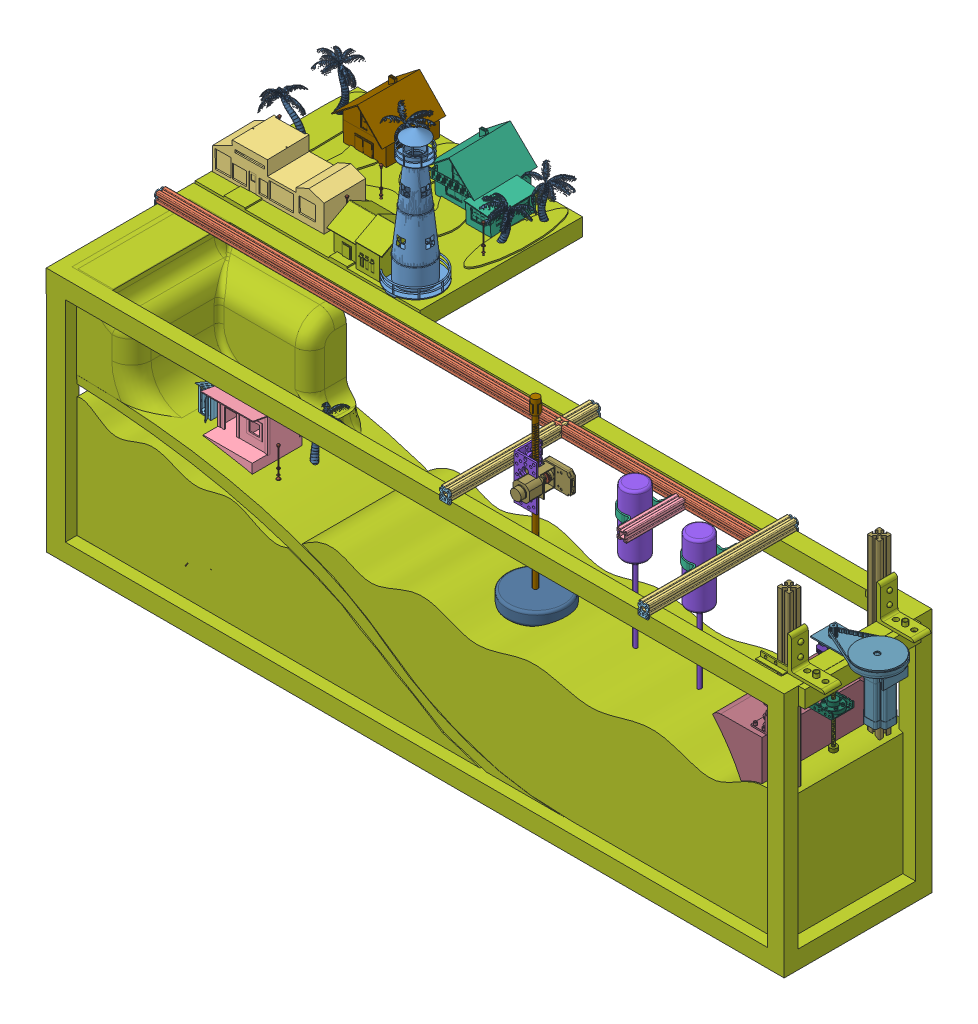
SolidWorks assembly Final SIWEED Town, configuration Default. Lengths in mm.
Overall size (1624.1 772.82 662.75).
56 component instances, 30 part files, 0 mates.
Components (placement in the parent):
- light house-1: light house [Valor predeterminado] at (-330.237 25.4911 -51.0609) size (102.96 270.27 102.96)
- tubular-seaweed-kcasal-2: tubular-seaweed-kcasal [Default] at (-568.4367 -469.1582 111.9112) size (107.7 163.84 96.86)
- tubular-seaweed-kcasal-3: tubular-seaweed-kcasal [Default] at (-442.6815 -467.3652 229.756) size (107.7 163.84 96.86)
- tubular-seaweed-kcasal-4: tubular-seaweed-kcasal [Default] at (-296.4049 -473.2054 80.9751) size (107.7 163.84 96.86)
- tubular-seaweed-kcasal-5: tubular-seaweed-kcasal [Default] at (-160.677 -471.1425 214.4198) size (107.7 163.84 96.86)
- tubular-seaweed-kcasal-6: tubular-seaweed-kcasal [Default] at (540.6521 -478.2942 227.6223) size (107.7 163.84 96.86)
- tubular-seaweed-kcasal-7: tubular-seaweed-kcasal [Default] at (365.184 -475.0345 56.2717) size (107.7 163.84 96.86)
- tubular-seaweed-kcasal-8: tubular-seaweed-kcasal [Default] at (621.9216 -477.4305 81.786) size (107.7 163.84 96.86)
- House-3: House [Default] at (-725.2491 24.3471 -33.5795) x (0.999899 0.000267 -0.014208) z (0.014208 -0.003565 0.999893) size (223.52 75.83 86.06)
- beach shack-1: beach shack [Default] at (-470.8744 -176.6109 240.0196) size (106.25 98.8 105.39)
- Outhouse-Open-2: Outhouse-Open [Default] at (-483.2149 -182.3943 199.9121) size (31.5 57.98 45.65)
- Countryside house-1: Countryside house [Default] at (-376.1849 -10.3567 -251.8498) x (-0.99973 -0.022381 0.006286) z (-0.02228 0.999628 0.015732) size (147.6 136.12 97.35)
- LH house-1: LH house [Default] at (-460.7063 23.119 -18.1219) size (112.96 74.71 94.82)
- wave measure-1: wave measure [Default] at (627.8869 73.115 135.3685) size (50 370 50)
- blue house 2 - Copy-1: blue house 2 - Copy [Default] at (-560.7085 -9.4422 -248.2312) x (-0.999775 -0.018539 -0.0103) z (-0.018603 0.999808 0.006151) size (106.85 125.4 97.89)
- palm tree-1: palm tree [Default] at (-704.5489 19.3291 -266.6541) x (0.815115 -0.579296 0.00211) z (-0.044941 -0.059603 0.99721) size (92.97 107.72 85.28)
- palm tree-2: palm tree [Default] at (-287.994 -4.5544 -294.1855) x (-0.657778 -0.58831 0.470339) z (-0.582054 0.000691 -0.81315) size (92.97 107.72 85.28)
- palm tree-3: palm tree [Default] at (-683.3902 -3.1186 -179.254) size (92.97 107.72 85.28)
- palm tree-4: palm tree [Default] at (-507.0238 19.3209 -256.8631) x (-0.527872 -0.751917 0.394933) z (-0.659035 0.069312 -0.748911) size (92.97 107.72 85.28)
- palm tree-5: palm tree [Default] at (-316.3627 -2.4735 -185.7607) x (-0.077598 -0.610207 -0.788433) z (0.965586 -0.242903 0.092961) size (92.97 107.72 85.28)
- palm tree-6: palm tree [Default] at (-328.8643 -222.7923 154.666) x (-0.799875 -0.565941 -0.199779) z (0.375561 -0.212342 -0.902144) size (92.97 107.72 85.28)
- Street light-1: Street light [Default] at (-504.7254 25.0065 -155.9439) size (7.68 64.16 7.68)
- Street light-2: Street light [Default] at (-695.218 24.2439 -139.581) size (7.68 64.16 7.68)
- Street light-3: Street light [Default] at (-300.9409 24.1249 -160.1755) size (7.68 64.16 7.68)
- Street light-4: Street light [Default] at (-485.6592 23.8662 -67.4403) size (7.68 64.16 7.68)
- Street light-5: Street light [Default] at (-342.5209 -201.1323 215.0846) size (7.68 64.16 7.68)
- Rod-2: Rod [Default] at (722.2608 -445.8472 240.2952) x (-0.004967 0 -0.999988) z (0.999988 0 -0.004967) size (25.05 603.25 29.28)
- Rod-3: Rod [Default] at (721.8173 -446.1515 56.2491) x (0.003725 0 -0.999993) z (0.999993 0 0.003725) size (25.05 603.25 29.28)
- FinalWaveMaker-1: FinalWaveMaker [Default] at (559.6345 -220.1914 268.4092) x (-0.007161 0 -0.999974) z (0.999974 0 -0.007161) size (248 243.14 114.31)
- Pulley-1: Pulley [Default] at (790.1881 26.1713 117.0535) x (-0.002142 0 -0.999998) z (0.999998 0 -0.002142) size (90 122.17 158.38)
- U Bracket-1: U Bracket [Default] at (683.6186 -106.2815 154.6387) x (-0.999989 0 0.004594) z (-0.004594 0 -0.999989) size (80 18 45)
- Long screw-1: Long screw [Default] at (720.8979 -177.7051 147.5263) size (14.81 201.01 14.81)
- Encoder-1: Encoder [Default] at (724.347 18.4275 145.9065) x (-0.00011 0.00348 0.999994) z (-0.00349 -0.999988 0.00348) size (36.76 27.38 12.49)
- Horiz Rod-2: Horiz Rod [Default] at (727.2348 -437.5203 233.7025) x (0.999978 0.006485 -0.001124) z (-0.006487 0.999977 -0.002044) size (25.05 165.17 25.02)
- mini bracket-1: mini bracket [Default] at (711.0813 -423.1445 184.1085) x (-0.022509 0 -0.999747) z (0.999747 0 -0.022509) size (38.1 41.91 21.59)
- mini bracket-2: mini bracket [Default] at (735.3926 -423.5938 119.6473) x (-0.008692 0 0.999962) z (-0.999962 0 -0.008692) size (38.1 41.91 21.59)
- Top Rods-1: Top Rods [Default] at (-882.7836 26.3586 62.697) x (-0.001829 -0.999998 0) z (0 0 1) size (20.13 1208 20.13)
- short Top Rods - -1: short Top Rods -  [Default] at (488.8957 26.1825 337.0082) x (1 0 0) z (0 1 0.000476) size (20.13 300 20.13)
- short Top Rods - -2: short Top Rods -  [Default] at (85.9161 26.5245 336.3662) x (1 0 0) z (0 0.999999 -0.001242) size (20.13 300 20.13)
- double S Top Rods -  - Copy-1: double S Top Rods -  - Copy [Default] at (336.8077 24.8488 207.6377) x (1 0 0) z (0 1 0.000493) size (20.13 120 20.13)
- rod connector-1: rod connector [Default] at (94.5354 20.9235 299.1846) size (21.59 25.4 2.54)
- rod connector-2: rod connector [Default] at (94.7649 20.5166 -3.7046) size (21.59 25.4 2.54)
- rod connector-3: rod connector [Default] at (497.9897 20.6321 299.4942) size (21.59 25.4 2.54)
- rod connector-4: rod connector [Default] at (498.1252 20.9408 -3.0849) size (21.59 25.4 2.54)
- rod connector-5: rod connector [Default] at (-734.5368 22.2519 52.3516) x (-0.013846 0 -0.999904) z (0.999904 0 -0.013846) size (21.59 25.4 2.54)
- wave brace-1: wave brace [Default] at (458.4496 20.4118 158.4076) size (51.5 15 106.34)
- wave brace-2: wave brace [Default] at (306.3657 19.3798 138.6013) size (51.5 15 106.34)
- wave measure-2: wave measure [Default] at (477.6178 74.3397 115.4999) size (50 370 50)
- Town Base-1: Town Base [Default] at (2.5968 -0.8548 -0.7979) size (1542.41 570 630.33)
- Buoy Part-1: Buoy Part [Default] at (160.9969 96.3447 60.8675) size (120 386.3 120)
  - bracket-1: bracket [Default] at (-39.1894 -173.2482 85.6941) size (45.72 91.44 45.72)
  - whole buoy prt-1: whole buoy prt [Default] at (-38.699 -299.0576 84.1766) size (18.22 341 17.87)
  - Final buoy-1: Final buoy [Default] at (-47.6966 -301.3654 85.301) size (120 50 120)
  - complete motor-1: complete motor [Default] at (-77.6982 -124.1154 -74.2161) size (57.88 41.08 90.03)
    - gear-1: gear [Default] at (79.9405 42.9351 181.082) x (0.002954 -0.001289 0.999995) z (0.566866 -0.823805 -0.002737) size (3.51 18.21 18.23)
    - Motor-1: Motor [Default] at (46.693 23.9348 130.7298) size (57.88 41.08 90.03)
